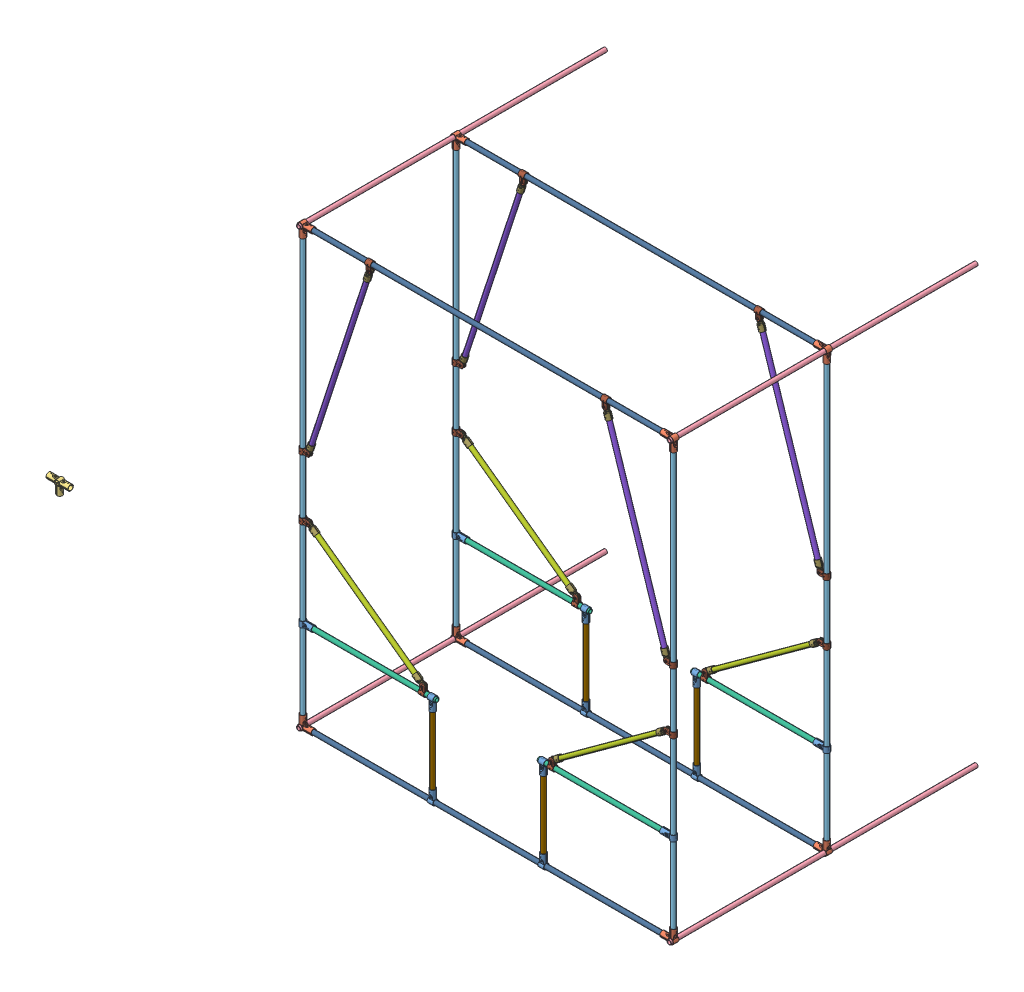
SolidWorks assembly SteelTubeAssembly, configuration Default. Lengths in mm.
Overall size (3684.85 2626.23 1877.32).
97 component instances, 12 part files, 70 mates.
Components (placement in the parent):
- 2534T210_CLAMP-ON FRAMING FITTING-2: 2534T210_CLAMP-ON FRAMING FITTING [2534T21] at (736.6 0 0) x (1 0 0) z (0 0 -1) size (33.53 82.55 34.1)
- 2534T240_CLAMP-ON FRAMING FITTING-1: 2534T240_CLAMP-ON FRAMING FITTING [2534T24] at (2171.7 0 0) x (-1 0 0) z (0 0 1) size (81.85 81.28 33.46)
- 2534T260_CLAMP-ON FRAMING FITTING-1: 2534T260_CLAMP-ON FRAMING FITTING [2534T26] at (-1430.376 594.6399 57.1912) size (130.05 82.36 33.46)
- Depth Bar-1: Depth Bar [Default] at (-38.1 0 -1803.4) x (0 0 1) z (-1 0 0) size (1828.8 25.4 25.4)
- Height-1: Height [Default] at (2171.7 2552.7 0) x (0 -1 0) z (-0.85323 0 -0.521535) size (2514.6 25.4 25.4)
- Horizonal Corner-1: Horizonal Corner [Default] at (0 533.4 0) x (1 0 0) z (0 0.49668 0.867934) size (762 25.4 25.4)
- Lower Mounting Bar-1: Lower Mounting Bar [Default] at (37.4552 1037.0521 0) x (0.809017 -0.587785 0) z (0.370288 0.509658 0.776618) size (762 25.4 25.4)
- Upper Mounting Bar-1: Upper Mounting Bar [Default] at (7.9592 1459.4984 0) x (0.309017 0.951057 0) z (0.948348 -0.308137 -0.075413) size (1117.6 25.4 25.4)
- Vertical Corner-1: Vertical Corner [Default] at (736.6 495.3 0) x (0 -1 0) z (-0.989698 0 0.143171) size (457.2 25.4 25.4)
- Width-1: Width [Default] at origin size (2133.6 25.4 25.4)
- 2534T240_CLAMP-ON FRAMING FITTING-2: 2534T240_CLAMP-ON FRAMING FITTING [2534T24] at (2171.7 2590.8 0) x (-1 0 0) z (0 0 -1) size (81.85 81.28 33.46)
- 2534T240_CLAMP-ON FRAMING FITTING-5: 2534T240_CLAMP-ON FRAMING FITTING [2534T24] at (-38.1 0 0) x (1 0 0) z (0 0 -1) size (81.85 81.28 33.46)
- Height-3: Height [Default] at (-38.1 2552.7 0) x (0 -1 0) z (-0.845396 0 -0.534139) size (2514.6 25.4 25.4)
- 2534T240_CLAMP-ON FRAMING FITTING-6: 2534T240_CLAMP-ON FRAMING FITTING [2534T24] at (-38.1 2590.8 0) size (81.85 81.28 33.46)
- Width-3: Width [Default] at (0 2590.8 0) x (1 0 0) z (0 0.262637 0.964895) size (2133.6 25.4 25.4)
- 2534T210_CLAMP-ON FRAMING FITTING-3: 2534T210_CLAMP-ON FRAMING FITTING [2534T21] at (736.6 533.4 0) size (33.53 82.55 34.1)
- 2534T210_CLAMP-ON FRAMING FITTING-5: 2534T210_CLAMP-ON FRAMING FITTING [2534T21] at (-38.1 533.4 0) x (0 -1 0) z (0 0 -1) size (33.53 82.55 34.1)
- 2534T210_CLAMP-ON FRAMING FITTING-10: 2534T210_CLAMP-ON FRAMING FITTING [2534T21] at (1397 0 0) x (1 0 0) z (0 0 -1) size (33.53 82.55 34.1)
- 2534T210_CLAMP-ON FRAMING FITTING-11: 2534T210_CLAMP-ON FRAMING FITTING [2534T21] at (1397 533.4 0) x (-1 0 0) z (0 0 -1) size (33.53 82.55 34.1)
- Vertical Corner-3: Vertical Corner [Default] at (1397 495.3 0) x (0 -1 0) z (-0.962184 0 -0.272399) size (457.2 25.4 25.4)
- Horizonal Corner-3: Horizonal Corner [Default] at (1371.6 533.4 0) x (1 0 0) z (0 -0.195703 0.980663) size (762 25.4 25.4)
- 2534T210_CLAMP-ON FRAMING FITTING-12: 2534T210_CLAMP-ON FRAMING FITTING [2534T21] at (2171.7 533.4 0) x (0 -1 0) z (0 0 1) size (33.53 82.55 34.1)
- Adjustable_18deg-1: Adjustable_18deg [Default] at (32.4607 1398.2418 -8.9201) size (87.05 82.3 33.53)
  - Adjustable Connector Part 1-1: Adjustable Connector Part 1 [2534T33] at (-70.5607 28.1617 8.9201) size (68.33 33.53 33.53)
  - Adjustable Connector Part 2-1: Adjustable Connector Part 2 [2534T33] at (-46.1648 -5.4163 8.9201) x (0.309017 0.951057 0) z (0 0 1) size (75.66 33.46 33.53)
- Adjustable_36deg-1: Adjustable_36deg [Default] at (710.24 603.9607 -8.9201) x (0 1 0) z (0 0 1) size (101.88 80.88 33.53)
  - Adjustable Connector Part 1-1: Adjustable Connector Part 1 [2534T33] at (-70.5607 28.1617 8.9201) size (68.33 33.53 33.53)
  - Adjustable Connector Part 2-1: Adjustable Connector Part 2 [2534T33] at (-56.007 -0.4015 8.9201) x (0.587785 0.809017 0) z (0 0 1) size (75.66 33.46 33.53)
- Adjustable_54deg-1: Adjustable_54deg [Default] at (32.4607 1094.4566 8.9201) x (1 0 0) z (0 0 -1) size (111.84 71.54 33.53)
  - Adjustable Connector Part 1-1: Adjustable Connector Part 1 [2534T33] at (-70.5607 28.1617 8.9201) size (68.33 33.53 33.53)
  - Adjustable Connector Part 2-1: Adjustable Connector Part 2 [2534T33] at (-63.8178 7.4093 8.9201) x (0.809017 0.587785 0) z (0 0 1) size (75.66 33.46 33.53)
- Adjustable_72deg-1: Adjustable_72deg [Default] at (392.2314 2520.2393 8.9201) x (0 -1 0) z (0 0 -1) size (115.94 55.2 33.53)
  - Adjustable Connector Part 1-1: Adjustable Connector Part 1 [2534T33] at (-70.5607 28.1617 8.9201) size (68.33 33.53 33.53)
  - Adjustable Connector Part 2-1: Adjustable Connector Part 2 [2534T33] at (-68.8327 17.2515 8.9201) x (0.951057 0.309017 0) z (0 0 1) size (75.66 33.46 33.53)
- Adjustable_72deg-2: Adjustable_72deg [Default] at (1741.3686 2520.2393 -8.9201) x (0 -1 0) z (0 0 1) size (115.94 55.2 33.53)
  - Adjustable Connector Part 1-1: Adjustable Connector Part 1 [2534T33] at (-70.5607 28.1617 8.9201) size (68.33 33.53 33.53)
  - Adjustable Connector Part 2-1: Adjustable Connector Part 2 [2534T33] at (-68.8327 17.2515 8.9201) x (0.951057 0.309017 0) z (0 0 1) size (75.66 33.46 33.53)
- Upper Mounting Bar-2: Upper Mounting Bar [Default] at (2125.6408 1459.4984 0) x (-0.309017 0.951057 0) z (0.948348 0.308137 0.075413) size (1117.6 25.4 25.4)
- Adjustable_18deg-2: Adjustable_18deg [Default] at (2101.1393 1398.2418 8.9201) x (-1 0 0) z (0 0 -1) size (87.05 82.3 33.53)
  - Adjustable Connector Part 1-1: Adjustable Connector Part 1 [2534T33] at (-70.5607 28.1617 8.9201) size (68.33 33.53 33.53)
  - Adjustable Connector Part 2-1: Adjustable Connector Part 2 [2534T33] at (-46.1648 -5.4163 8.9201) x (0.309017 0.951057 0) z (0 0 1) size (75.66 33.46 33.53)
- Adjustable_36deg-2: Adjustable_36deg [Default] at (1423.36 603.9607 8.9201) x (0 1 0) z (0 0 -1) size (101.88 80.88 33.53)
  - Adjustable Connector Part 1-1: Adjustable Connector Part 1 [2534T33] at (-70.5607 28.1617 8.9201) size (68.33 33.53 33.53)
  - Adjustable Connector Part 2-1: Adjustable Connector Part 2 [2534T33] at (-56.007 -0.4015 8.9201) x (0.587785 0.809017 0) z (0 0 1) size (75.66 33.46 33.53)
- Lower Mounting Bar-2: Lower Mounting Bar [Default] at (2096.1448 1037.0521 0) x (-0.809017 -0.587785 0) z (0.370288 -0.509658 -0.776618) size (762 25.4 25.4)
- Adjustable_54deg-2: Adjustable_54deg [Default] at (2101.1393 1094.4566 -8.9201) x (-1 0 0) z (0 0 1) size (111.84 71.54 33.53)
  - Adjustable Connector Part 1-1: Adjustable Connector Part 1 [2534T33] at (-70.5607 28.1617 8.9201) size (68.33 33.53 33.53)
  - Adjustable Connector Part 2-1: Adjustable Connector Part 2 [2534T33] at (-63.8178 7.4093 8.9201) x (0.809017 0.587785 0) z (0 0 1) size (75.66 33.46 33.53)
- Width-4: Width [Default] at (0 2590.8 -914.4) x (1 0 0) z (0 -0.262637 0.964895) size (2133.6 25.4 25.4)
- Height-4: Height [Default] at (-38.1 2552.7 -914.4) x (0 -1 0) z (0.845396 0 -0.534139) size (2514.6 25.4 25.4)
- 2534T240_CLAMP-ON FRAMING FITTING-7: 2534T240_CLAMP-ON FRAMING FITTING [2534T24] at (-38.1 2590.8 -914.4) size (81.85 81.28 33.46)
- Upper Mounting Bar-3: Upper Mounting Bar [Default] at (7.9592 1459.4984 -914.4) x (0.309017 0.951057 0) z (-0.948348 0.308137 -0.075413) size (1117.6 25.4 25.4)
- Adjustable_72deg-3: Adjustable_72deg [Default] at (392.2314 2520.2393 -905.4799) x (0 -1 0) z (0 0 -1) size (115.94 55.2 33.53)
  - Adjustable Connector Part 1-1: Adjustable Connector Part 1 [2534T33] at (-70.5607 28.1617 8.9201) size (68.33 33.53 33.53)
  - Adjustable Connector Part 2-1: Adjustable Connector Part 2 [2534T33] at (-68.8327 17.2515 8.9201) x (0.951057 0.309017 0) z (0 0 1) size (75.66 33.46 33.53)
- Adjustable_54deg-3: Adjustable_54deg [Default] at (32.4607 1094.4566 -905.4799) x (1 0 0) z (0 0 -1) size (111.84 71.54 33.53)
  - Adjustable Connector Part 1-1: Adjustable Connector Part 1 [2534T33] at (-70.5607 28.1617 8.9201) size (68.33 33.53 33.53)
  - Adjustable Connector Part 2-1: Adjustable Connector Part 2 [2534T33] at (-63.8178 7.4093 8.9201) x (0.809017 0.587785 0) z (0 0 1) size (75.66 33.46 33.53)
- Adjustable_18deg-3: Adjustable_18deg [Default] at (32.4607 1398.2418 -923.3201) size (87.05 82.3 33.53)
  - Adjustable Connector Part 1-1: Adjustable Connector Part 1 [2534T33] at (-70.5607 28.1617 8.9201) size (68.33 33.53 33.53)
  - Adjustable Connector Part 2-1: Adjustable Connector Part 2 [2534T33] at (-46.1648 -5.4163 8.9201) x (0.309017 0.951057 0) z (0 0 1) size (75.66 33.46 33.53)
- Lower Mounting Bar-3: Lower Mounting Bar [Default] at (37.4552 1037.0521 -914.4) x (0.809017 -0.587785 0) z (-0.370288 -0.509658 0.776618) size (762 25.4 25.4)
- Horizonal Corner-4: Horizonal Corner [Default] at (0 533.4 -914.4) x (1 0 0) z (0 -0.49668 0.867934) size (762 25.4 25.4)
- 2534T210_CLAMP-ON FRAMING FITTING-13: 2534T210_CLAMP-ON FRAMING FITTING [2534T21] at (-38.1 533.4 -914.4) x (0 1 0) z (0 0 1) size (33.53 82.55 34.1)
- Adjustable_36deg-3: Adjustable_36deg [Default] at (710.24 603.9607 -923.3201) x (0 1 0) z (0 0 1) size (101.88 80.88 33.53)
  - Adjustable Connector Part 1-1: Adjustable Connector Part 1 [2534T33] at (-70.5607 28.1617 8.9201) size (68.33 33.53 33.53)
  - Adjustable Connector Part 2-1: Adjustable Connector Part 2 [2534T33] at (-56.007 -0.4015 8.9201) x (0.587785 0.809017 0) z (0 0 1) size (75.66 33.46 33.53)
- Vertical Corner-4: Vertical Corner [Default] at (736.6 495.3 -914.4) x (0 -1 0) z (0.989698 0 0.143171) size (457.2 25.4 25.4)
- 2534T210_CLAMP-ON FRAMING FITTING-14: 2534T210_CLAMP-ON FRAMING FITTING [2534T21] at (736.6 533.4 -914.4) x (-1 0 0) z (0 0 -1) size (33.53 82.55 34.1)
- Width-5: Width [Default] at (0 0 -914.4) size (2133.6 25.4 25.4)
- 2534T240_CLAMP-ON FRAMING FITTING-8: 2534T240_CLAMP-ON FRAMING FITTING [2534T24] at (-38.1 0 -914.4) x (1 0 0) z (0 0 -1) size (81.85 81.28 33.46)
- Adjustable_54deg-4: Adjustable_54deg [Default] at (2101.1393 1094.4566 -923.3201) x (-1 0 0) z (0 0 1) size (111.84 71.54 33.53)
  - Adjustable Connector Part 1-1: Adjustable Connector Part 1 [2534T33] at (-70.5607 28.1617 8.9201) size (68.33 33.53 33.53)
  - Adjustable Connector Part 2-1: Adjustable Connector Part 2 [2534T33] at (-63.8178 7.4093 8.9201) x (0.809017 0.587785 0) z (0 0 1) size (75.66 33.46 33.53)
- Lower Mounting Bar-4: Lower Mounting Bar [Default] at (2096.1448 1037.0521 -914.4) x (-0.809017 -0.587785 0) z (-0.370288 0.509658 -0.776618) size (762 25.4 25.4)
- Upper Mounting Bar-4: Upper Mounting Bar [Default] at (2125.6408 1459.4984 -914.4) x (-0.309017 0.951057 0) z (-0.948348 -0.308137 0.075413) size (1117.6 25.4 25.4)
- Adjustable_36deg-4: Adjustable_36deg [Default] at (1423.36 603.9607 -905.4799) x (0 1 0) z (0 0 -1) size (101.88 80.88 33.53)
  - Adjustable Connector Part 1-1: Adjustable Connector Part 1 [2534T33] at (-70.5607 28.1617 8.9201) size (68.33 33.53 33.53)
  - Adjustable Connector Part 2-1: Adjustable Connector Part 2 [2534T33] at (-56.007 -0.4015 8.9201) x (0.587785 0.809017 0) z (0 0 1) size (75.66 33.46 33.53)
- Adjustable_18deg-4: Adjustable_18deg [Default] at (2101.1393 1398.2418 -905.4799) x (-1 0 0) z (0 0 -1) size (87.05 82.3 33.53)
  - Adjustable Connector Part 1-1: Adjustable Connector Part 1 [2534T33] at (-70.5607 28.1617 8.9201) size (68.33 33.53 33.53)
  - Adjustable Connector Part 2-1: Adjustable Connector Part 2 [2534T33] at (-46.1648 -5.4163 8.9201) x (0.309017 0.951057 0) z (0 0 1) size (75.66 33.46 33.53)
- Adjustable_72deg-4: Adjustable_72deg [Default] at (1741.3686 2520.2393 -923.3201) x (0 -1 0) z (0 0 1) size (115.94 55.2 33.53)
  - Adjustable Connector Part 1-1: Adjustable Connector Part 1 [2534T33] at (-70.5607 28.1617 8.9201) size (68.33 33.53 33.53)
  - Adjustable Connector Part 2-1: Adjustable Connector Part 2 [2534T33] at (-68.8327 17.2515 8.9201) x (0.951057 0.309017 0) z (0 0 1) size (75.66 33.46 33.53)
- 2534T210_CLAMP-ON FRAMING FITTING-15: 2534T210_CLAMP-ON FRAMING FITTING [2534T21] at (1397 0 -913.8268) x (1 0 0) z (0 0 -1) size (33.53 82.55 34.1)
- 2534T210_CLAMP-ON FRAMING FITTING-16: 2534T210_CLAMP-ON FRAMING FITTING [2534T21] at (2171.7 533.4 -914.4) x (0 1 0) z (0 0 -1) size (33.53 82.55 34.1)
- Horizonal Corner-5: Horizonal Corner [Default] at (1371.6 533.4 -914.4) x (1 0 0) z (0 0.195703 0.980663) size (762 25.4 25.4)
- Vertical Corner-5: Vertical Corner [Default] at (1397 495.3 -914.4) x (0 -1 0) z (0.962184 0 -0.272399) size (457.2 25.4 25.4)
- 2534T210_CLAMP-ON FRAMING FITTING-17: 2534T210_CLAMP-ON FRAMING FITTING [2534T21] at (1397 533.4 -913.8268) x (-1 0 0) z (0 0 -1) size (33.53 82.55 34.1)
- 2534T240_CLAMP-ON FRAMING FITTING-9: 2534T240_CLAMP-ON FRAMING FITTING [2534T24] at (2171.7 2590.8 -914.4) x (-1 0 0) z (0 0 -1) size (81.85 81.28 33.46)
- 2534T210_CLAMP-ON FRAMING FITTING-18: 2534T210_CLAMP-ON FRAMING FITTING [2534T21] at (736.6 0 -913.8268) x (1 0 0) z (0 0 -1) size (33.53 82.55 34.1)
- 2534T240_CLAMP-ON FRAMING FITTING-10: 2534T240_CLAMP-ON FRAMING FITTING [2534T24] at (2171.7 0 -914.4) x (-1 0 0) z (0 0 1) size (81.85 81.28 33.46)
- Height-5: Height [Default] at (2171.7 2552.7 -914.4) x (0 -1 0) z (0.85323 0 -0.521535) size (2514.6 25.4 25.4)
- Depth Bar-2: Depth Bar [Default] at (2171.7 0 25.4) x (0 0 -1) z (0.840422 0.541932 0) size (1828.8 25.4 25.4)
- Depth Bar-3: Depth Bar [Default] at (-38.1 2590.8 25.4) x (0 0 -1) z (-0.633686 -0.77359 0) size (1828.8 25.4 25.4)
- Depth Bar-4: Depth Bar [Default] at (2171.7 2590.8 -1803.4) x (0 0 1) z (-0.806438 -0.591319 0) size (1828.8 25.4 25.4)
Mates (geometry in assembly coordinates):
- Coincident1: coordinate: point of Width-1; point of assembly
- Concentric1: concentric anti-aligned: cylinder of 2534T240_CLAMP-ON FRAMING FITTING-1 through (2107.184 0 0) axis (1 0 0) radius 13.97; cylinder of Width-1 through (2133.6 0 0) axis (-1 0 0) radius 12.7
- Distance1: distance = 38.1 mm: point of 2534T240_CLAMP-ON FRAMING FITTING-1; plane of Width-1 through (2133.6 0 0) normal (1 0 0)
- Coincident2: coincident aligned: plane of Width-1 through (0 0 0) normal (0 0 1); plane of assembly through (0 0 0) normal (0 0 1)
- Parallel1: parallel aligned: plane of 2534T240_CLAMP-ON FRAMING FITTING-1 through (2171.7 64.516 0) normal (0 1 0); plane of assembly through (0 0 0) normal (0 1 0)
- Concentric2: concentric anti-aligned: cylinder of 2534T240_CLAMP-ON FRAMING FITTING-1 through (2171.7 64.516 0) axis (0 -1 0) radius 13.97; cylinder of Height-1 through (2171.7 38.1 0) axis (0 1 0) radius 12.7
- Distance2: distance = 38.1 mm anti-aligned: plane of Height-1 through (2171.7 38.1 0) normal (0 -1 0); plane of Width-1 through (0 0 0) normal (0 1 0)
- Concentric3: concentric aligned: cylinder of Height-1 through (2171.7 38.1 0) axis (0 1 0) radius 12.7; cylinder of 2534T240_CLAMP-ON FRAMING FITTING-2 through (2171.7 2526.284 0) axis (0 1 0) radius 13.97
- Distance3: distance = 38.1 mm: plane of Height-1 through (2171.7 2552.7 0) normal (0 1 0); point of 2534T240_CLAMP-ON FRAMING FITTING-2
- Parallel2: parallel aligned: plane of 2534T240_CLAMP-ON FRAMING FITTING-2 through (2171.7 2590.8 16.73) normal (0 0 1); plane of assembly through (0 0 0) normal (0 0 1)
- Concentric13: concentric aligned: cylinder of Width-1 through (2133.6 0 0) axis (-1 0 0) radius 12.7; cylinder of 2534T240_CLAMP-ON FRAMING FITTING-5 through (26.416 0 0) axis (-1 0 0) radius 13.97
- Distance9: distance = 38.1 mm: plane of Width-1 through (0 0 0) normal (-1 0 0); point of 2534T240_CLAMP-ON FRAMING FITTING-5
- Parallel5: parallel aligned: plane of 2534T240_CLAMP-ON FRAMING FITTING-1 through (2171.7 64.516 0) normal (0 1 0); plane of 2534T240_CLAMP-ON FRAMING FITTING-5 through (-38.1 64.516 0) normal (0 1 0)
- Concentric14: concentric anti-aligned: cylinder of 2534T240_CLAMP-ON FRAMING FITTING-5 through (-38.1 64.516 0) axis (0 -1 0) radius 13.97; cylinder of Height-3 through (-38.1 38.1 0) axis (0 1 0) radius 12.7
- Distance10: distance = 38.1 mm: plane of Height-3 through (-38.1 38.1 0) normal (0 -1 0); point of 2534T240_CLAMP-ON FRAMING FITTING-5
- Concentric15: concentric aligned: cylinder of Height-3 through (-38.1 38.1 0) axis (0 1 0) radius 12.7; cylinder of 2534T240_CLAMP-ON FRAMING FITTING-6 through (-38.1 2526.284 0) axis (0 1 0) radius 13.97
- Distance11: distance = 38.1 mm: plane of Height-3 through (-38.1 2552.7 0) normal (0 1 0); point of 2534T240_CLAMP-ON FRAMING FITTING-6
- Parallel6: parallel aligned: plane of Height-1 through (2171.7 2552.7 0) normal (0 1 0); plane of Height-3 through (-38.1 2552.7 0) normal (0 1 0)
- Concentric16: concentric anti-aligned: cylinder of 2534T240_CLAMP-ON FRAMING FITTING-2 through (2107.184 2590.8 0) axis (1 0 0) radius 13.97; cylinder of Width-3 through (2133.6 2590.8 0) axis (-1 0 0) radius 12.7
- Distance12: distance = 38.1 mm: point of 2534T240_CLAMP-ON FRAMING FITTING-2; plane of Width-3 through (2133.6 2590.8 0) normal (1 0 0)
- Parallel8: parallel anti-aligned: plane of 2534T240_CLAMP-ON FRAMING FITTING-2 through (2107.184 2590.8 0) normal (-1 0 0); plane of 2534T240_CLAMP-ON FRAMING FITTING-6 through (26.416 2590.8 0) normal (1 0 0)
- Concentric19: concentric aligned: cylinder of 2534T210_CLAMP-ON FRAMING FITTING-2 through (753.364 0 0) axis (-1 0 0) radius 13.97; cylinder of Width-1 through (2133.6 0 0) axis (-1 0 0) radius 12.7
- Parallel9: parallel aligned: plane of 2534T210_CLAMP-ON FRAMING FITTING-2 through (736.6 65.786 0) normal (0 1 0); plane of 2534T240_CLAMP-ON FRAMING FITTING-5 through (-38.1 64.516 0) normal (0 1 0)
- Concentric20: concentric anti-aligned: cylinder of 2534T210_CLAMP-ON FRAMING FITTING-2 through (736.6 65.786 0) axis (0 -1 0) radius 13.97; cylinder of Vertical Corner-1 through (736.6 38.1 0) axis (0 1 0) radius 12.7
- Distance13: distance = 38.1 mm: point of 2534T210_CLAMP-ON FRAMING FITTING-2; plane of Vertical Corner-1 through (736.6 38.1 0) normal (0 -1 0)
- Concentric24: concentric aligned: cylinder of Vertical Corner-1 through (736.6 38.1 0) axis (0 1 0) radius 12.7; cylinder of 2534T210_CLAMP-ON FRAMING FITTING-3 through (736.6 467.614 0) axis (0 1 0) radius 13.97
- Distance14: distance = 38.1 mm: point of 2534T210_CLAMP-ON FRAMING FITTING-3; plane of Vertical Corner-1 through (736.6 495.3 0) normal (0 1 0)
- Concentric25: concentric anti-aligned: cylinder of Height-3 through (-38.1 38.1 0) axis (0 1 0) radius 12.7; cylinder of 2534T210_CLAMP-ON FRAMING FITTING-5 through (-38.1 550.164 0) axis (0 -1 0) radius 13.97
- Parallel10: parallel aligned: plane of 2534T240_CLAMP-ON FRAMING FITTING-5 through (26.416 0 0) normal (1 0 0); plane of 2534T210_CLAMP-ON FRAMING FITTING-5 through (27.686 533.4 0) normal (1 0 0)
- Parallel11: parallel anti-aligned: plane of 2534T210_CLAMP-ON FRAMING FITTING-3 through (719.836 533.4 0) normal (-1 0 0); plane of 2534T210_CLAMP-ON FRAMING FITTING-5 through (27.686 533.4 0) normal (1 0 0)
- Concentric26: concentric aligned: cylinder of Horizonal Corner-1 through (762 533.4 0) axis (-1 0 0) radius 12.7; cylinder of 2534T210_CLAMP-ON FRAMING FITTING-3 through (753.364 533.4 0) axis (-1 0 0) radius 13.97
- Distance15: distance = 25.4 mm: point of 2534T210_CLAMP-ON FRAMING FITTING-3; plane of Horizonal Corner-1 through (762 533.4 0) normal (1 0 0)
- Distance16: distance = 38.1 mm: plane of Horizonal Corner-1 through (0 533.4 0) normal (-1 0 0); point of 2534T210_CLAMP-ON FRAMING FITTING-5
- Concentric27: concentric aligned: cylinder of Horizonal Corner-1 through (762 533.4 0) axis (-1 0 0) radius 12.7; cylinder of 2534T210_CLAMP-ON FRAMING FITTING-5 through (27.686 533.4 0) axis (-1 0 0) radius 13.97
- Concentric28: concentric aligned: cylinder of ? through (569.8292 2128.6091 5503.5233) axis (0 1 0) radius 12.7; cylinder of ? through (569.8292 2558.1231 5503.5233) axis (0 1 0) radius 13.97
- Distance17: distance = 25.4 mm: point of ?; plane of ? through (595.2292 2623.9091 5503.5233) normal (1 0 0)
- Distance19: distance = 38.1 mm: point of ?; plane of ? through (569.8292 2585.8091 5503.5233) normal (0 1 0)
- Concentric30: concentric aligned: cylinder of ? through (595.2292 2623.9091 5503.5233) axis (-1 0 0) radius 12.7; cylinder of ? through (586.5932 2623.9091 5503.5233) axis (-1 0 0) radius 13.97
- Concentric31: concentric anti-aligned: cylinder of Width-1 through (2133.6 0 0) axis (-1 0 0) radius 12.7; cylinder of 2534T210_CLAMP-ON FRAMING FITTING-10 through (1380.236 0 0) axis (1 0 0) radius 13.97
- Concentric32: concentric anti-aligned: cylinder of 2534T210_CLAMP-ON FRAMING FITTING-10 through (1397 65.786 0) axis (0 -1 0) radius 13.97; cylinder of Vertical Corner-3 through (1397 38.1 0) axis (0 1 0) radius 12.7
- Distance20: distance = 38.1 mm: plane of Vertical Corner-3 through (1397 38.1 0) normal (0 -1 0); point of 2534T210_CLAMP-ON FRAMING FITTING-10
- Concentric33: concentric aligned: cylinder of 2534T210_CLAMP-ON FRAMING FITTING-11 through (1397 467.614 0) axis (0 1 0) radius 13.97; cylinder of Vertical Corner-3 through (1397 38.1 0) axis (0 1 0) radius 12.7
- Parallel12: parallel aligned: plane of 2534T240_CLAMP-ON FRAMING FITTING-1 through (2171.7 64.516 0) normal (0 1 0); plane of Vertical Corner-3 through (1397 495.3 0) normal (0 1 0)
- Distance21: distance = 38.1 mm: point of 2534T210_CLAMP-ON FRAMING FITTING-11; plane of Vertical Corner-3 through (1397 495.3 0) normal (0 1 0)
- Parallel13: parallel anti-aligned: plane of 2534T210_CLAMP-ON FRAMING FITTING-3 through (753.364 533.4 0) normal (1 0 0); plane of 2534T210_CLAMP-ON FRAMING FITTING-11 through (1380.236 533.4 0) normal (-1 0 0)
- Concentric34: concentric aligned: cylinder of 2534T210_CLAMP-ON FRAMING FITTING-11 through (1413.764 533.4 0) axis (-1 0 0) radius 13.97; cylinder of Horizonal Corner-3 through (2133.6 533.4 0) axis (-1 0 0) radius 12.7
- Distance22: distance = 25.4 mm: point of 2534T210_CLAMP-ON FRAMING FITTING-11; plane of Horizonal Corner-3 through (1371.6 533.4 0) normal (-1 0 0)
- Concentric35: concentric anti-aligned: cylinder of Height-1 through (2171.7 38.1 0) axis (0 1 0) radius 12.7; cylinder of 2534T210_CLAMP-ON FRAMING FITTING-12 through (2171.7 550.164 0) axis (0 -1 0) radius 13.97
- Concentric36: concentric anti-aligned: cylinder of Horizonal Corner-3 through (2133.6 533.4 0) axis (-1 0 0) radius 12.7; cylinder of 2534T210_CLAMP-ON FRAMING FITTING-12 through (2105.914 533.4 0) axis (1 0 0) radius 13.97
- Distance23: distance = 38.1 mm: point of 2534T210_CLAMP-ON FRAMING FITTING-12; plane of Horizonal Corner-3 through (2133.6 533.4 0) normal (1 0 0)
- Concentric37: concentric aligned: cylinder of Height-3 through (-38.1 38.1 0) axis (0 1 0) radius 12.7; cylinder of Adjustable_18deg-1/Adjustable Connector Part 1-1 through (-38.1 1409.6385 0) axis (0 1 0) radius 13.97
- Concentric38: concentric anti-aligned: cylinder of Upper Mounting Bar-1 through (353.3166 2522.3991 0) axis (-0.309017 -0.951057 0) radius 12.7; cylinder of Adjustable_18deg-1/Adjustable Connector Part 2-1 through (4.0347 1447.42 0) axis (0.309017 0.951057 0) radius 13.97
- Concentric39: concentric aligned: cylinder of Width-3 through (2133.6 2590.8 0) axis (-1 0 0) radius 12.7; cylinder of Adjustable_72deg-1/Adjustable Connector Part 1-1 through (380.8347 2590.8 0) axis (-1 0 0) radius 13.97
- Concentric40: concentric aligned: cylinder of Upper Mounting Bar-1 through (353.3166 2522.3991 0) axis (-0.309017 -0.951057 0) radius 12.7; cylinder of Adjustable_72deg-1/Adjustable Connector Part 2-1 through (357.2411 2534.4776 0) axis (-0.309017 -0.951057 0) radius 13.97
- Distance24: distance = 12.7 mm: plane of Upper Mounting Bar-1 through (353.3166 2522.3991 0) normal (0.309017 0.951057 0); line of Adjustable_72deg-1 through (357.2411 2534.4776 -7.4998) axis (0 0 1)
- Distance27: distance = 1083.1165 mm anti-aligned: plane of Adjustable_18deg-1/Adjustable Connector Part 1-1 through (-38.1 1443.1675 0) normal (0 1 0); plane of 2534T240_CLAMP-ON FRAMING FITTING-6 through (-38.1 2526.284 0) normal (0 -1 0)
- Concentric41: concentric aligned: cylinder of Horizonal Corner-1 through (762 533.4 0) axis (-1 0 0) radius 12.7; cylinder of Adjustable_36deg-1/Adjustable Connector Part 1-1 through (698.8434 533.4 0) axis (-1 0 0) radius 13.97
- Concentric42: concentric anti-aligned: cylinder of Height-3 through (-38.1 38.1 0) axis (0 1 0) radius 12.7; cylinder of Adjustable_54deg-1/Adjustable Connector Part 1-1 through (-38.1 1083.0599 0) axis (0 -1 0) radius 13.97
- Concentric43: concentric anti-aligned: cylinder of Lower Mounting Bar-1 through (653.9262 589.1598 0) axis (-0.809017 0.587785 0) radius 12.7; cylinder of Adjustable_54deg-1/Adjustable Connector Part 2-1 through (15.0837 1053.306 0) axis (0.809017 -0.587785 0) radius 13.97
- Concentric44: concentric aligned: cylinder of Lower Mounting Bar-1 through (653.9262 589.1598 0) axis (-0.809017 0.587785 0) radius 12.7; cylinder of Adjustable_36deg-1/Adjustable Connector Part 2-1 through (664.2007 581.6949 0) axis (-0.809017 0.587785 0) radius 13.97
- Distance28: distance = 12.7 mm: plane of Lower Mounting Bar-1 through (653.9262 589.1598 0) normal (0.809017 -0.587785 0); line of Adjustable_36deg-1 through (664.2007 581.6949 7.4998) axis (0 0 -1)
- Distance30: distance = 499.3669 mm anti-aligned: plane of 2534T210_CLAMP-ON FRAMING FITTING-5 through (-38.1 550.164 0) normal (0 1 0); plane of Adjustable_54deg-1/Adjustable Connector Part 1-1 through (-38.1 1049.5309 0) normal (0 -1 0)
- Concentric45: concentric: cylinder of Depth Bar-1 through (-38.1 0 25.4) axis (0 0 -1) radius 12.7; cylinder of 2534T240_CLAMP-ON FRAMING FITTING-5 through (-38.1 0 -16.731) axis (0 0 1) radius 13.97
- Distance31: distance = 25.4 mm: plane of Depth Bar-1 through (-38.1 0 25.4) normal (0 0 1); point of 2534T240_CLAMP-ON FRAMING FITTING-5
- Concentric46: concentric: cylinder of 2534T240_CLAMP-ON FRAMING FITTING-2 through (2171.7 2590.8 -16.731) axis (0 0 1) radius 13.97; cylinder of Depth Bar-4 through (2171.7 2590.8 25.4) axis (0 0 -1) radius 12.7
- Concentric47: concentric: cylinder of 2534T240_CLAMP-ON FRAMING FITTING-1 through (2171.7 0 16.731) axis (0 0 -1) radius 13.97; cylinder of Depth Bar-2 through (2171.7 0 -1705.567) axis (0 0 1) radius 12.7
- Concentric48: concentric: cylinder of 2534T240_CLAMP-ON FRAMING FITTING-6 through (-38.1 2590.8 16.731) axis (0 0 -1) radius 13.97; cylinder of Depth Bar-3 through (-38.1 2590.8 -1803.4) axis (0 0 1) radius 12.7
- Distance32: distance = 25.4 mm: plane of Depth Bar-3 through (-38.1 2590.8 25.4) normal (0 0 1); point of 2534T240_CLAMP-ON FRAMING FITTING-6
- Distance33: distance = 25.4 mm: plane of Depth Bar-4 through (2171.7 2590.8 25.4) normal (0 0 1); point of 2534T240_CLAMP-ON FRAMING FITTING-2
- Distance34: distance = 25.4 mm: plane of Depth Bar-2 through (2171.7 0 25.4) normal (0 0 1); point of 2534T240_CLAMP-ON FRAMING FITTING-1
